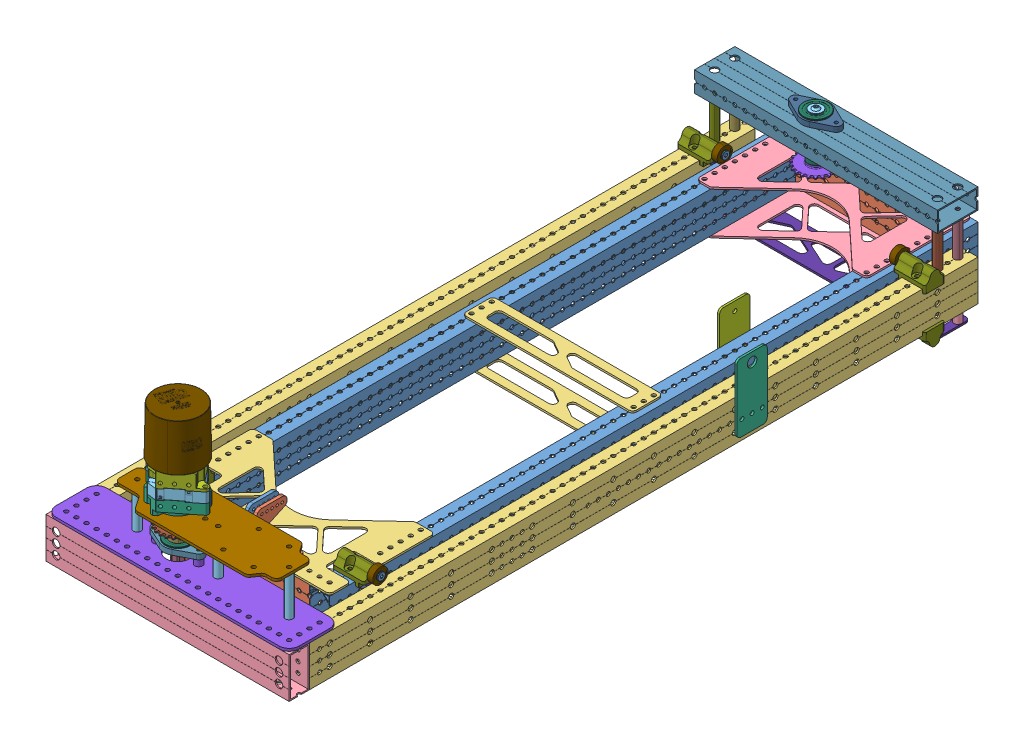
SolidWorks assembly Elevator Assembly 3.0, configuration Default. Lengths in mm. (continued)
Mates (geometry in assembly coordinates): (continued)
- Coincident51: coincident aligned: plane of WCP-EX-0018-001(2)^Assem1-1 through (-106.988 397.7257 1167.4134) normal (-1 0 0); plane of WCP-EX-0018-005(2)^Assem1-2 through (-106.988 397.7257 1116.6134) normal (-1 0 0)
- Distance1: distance = 12.7 mm anti-aligned: plane of WCP-EX-0018-005(2)^Assem1-1 through (172.412 397.7257 1116.6134) normal (-1 0 0); plane of 32inTubeStock-1 through (159.712 397.7257 265.7134) normal (1 0 0)
- Coincident53: coincident anti-aligned: plane of 32inTubeStock-1 through (159.712 448.5257 265.7134) normal (0 1 0); plane of Copy of WCP-0323 - Elevator Clamping Block-1-1/WCP-0323-001 Rev2^Copy of WCP-0323 - Elevator Clamping Block-1-1 through (159.7755 448.5257 1034.0634) normal (0 -1 0)
- Coincident57: coincident anti-aligned: plane of 7inRevTube-1 through (-43.488 448.5257 1053.1134) normal (0 1 0); plane of Inside_Bottom_Plate-1 through (-738.7858 448.5257 1008.0258) normal (0 -1 0)
- Concentric31: concentric anti-aligned: cylinder of 32inTubeStock-1 through (147.012 397.7257 1002.3134) axis (0 1 0) radius 2.5; cylinder of Inside_Bottom_Plate-1 through (147.012 450.8117 1002.3134) axis (0 -1 0) radius 2.4892
- Coincident59: coincident aligned: plane of 32inTubeStock-1 through (147.012 423.1257 1078.5134) normal (0 0 1); plane of Inside_Bottom_Plate-1 through (-738.7858 450.8117 1078.5134) normal (0 0 1)
- Concentric32: concentric anti-aligned: cylinder of 32inTubeStock-1 through (147.012 397.7257 1027.7134) axis (0 1 0) radius 2.5; cylinder of Copy of WCP-0323 - Elevator Clamping Block-1-1/WCP-0323-001 Rev2^Copy of WCP-0323 - Elevator Clamping Block-1-1 through (147.012 464.4007 1027.7134) axis (0 -1 0) radius 2.4892
- Concentric33: concentric anti-aligned: cylinder of 32inTubeStock-1 through (147.012 397.7257 1040.4134) axis (0 1 0) radius 2.5; cylinder of Copy of WCP-0323 - Elevator Clamping Block-1-1/WCP-0323-001 Rev2^Copy of WCP-0323 - Elevator Clamping Block-1-1 through (147.012 448.5257 1040.4134) axis (0 -1 0) radius 2.0193
- Concentric37: concentric anti-aligned: cylinder of 32inTubeStock-2 through (-56.188 397.7257 278.4134) axis (0 1 0) radius 2.5; cylinder of Inside_Top_Plate-1 through (-56.188 450.8117 278.4134) axis (0 -1 0) radius 2.4892
- Coincident65: coincident anti-aligned: plane of 7inRevTube-2 through (-43.488 448.5257 265.7134) normal (0 1 0); plane of Inside_Top_Plate-1 through (45.412 448.5257 384.432) normal (0 -1 0)
- Concentric38: concentric anti-aligned: cylinder of 32inTubeStock-1 through (147.012 397.7257 278.4134) axis (0 1 0) radius 2.5; cylinder of Inside_Top_Plate-1 through (147.012 450.8117 278.4134) axis (0 -1 0) radius 2.4892
- Concentric43: concentric anti-aligned: cylinder of Copy (2) of Copy of WCP-0571 Rev1^Elevator Assembly Updated 3.0-2 through (20.012 468.1632 329.2134) axis (0 1 0) radius 7.94; cylinder of Copy of Copy of WCP-0599 Rev1^Elevator Assembly Updated 3.0-1 through (20.012 469.1632 329.2134) axis (0 -1 0) radius 2.0193
- Concentric44: concentric anti-aligned: cylinder of Copy of Copy of WCP-0599 Rev1^Elevator Assembly Updated 3.0-1 through (20.012 469.1632 329.2134) axis (0 -1 0) radius 2.0193; cylinder of WCP-0790_500L_500_hex.step-1 through (20.012 478.6882 329.2134) axis (0 1 0) radius 9.75
- Concentric45: concentric anti-aligned: cylinder of Copy of Copy of WCP-0599 Rev1^Elevator Assembly 3.0-1 through (20.012 469.1632 329.2134) axis (0 -1 0) radius 2.0193; cylinder of Copy of Copy (2) of WCP-0560 Rev1^Elevator Assembly 3.0-1 through (20.012 469.1632 329.2134) axis (0 1 0) radius 9.525
- Concentric46: concentric aligned: unknown of Copy of Copy of WCP-0571 Rev1^Elevator Assembly Updated 3.0-1; cylinder of Copy of Copy of WCP-0599 Rev1^Elevator Assembly Updated 3.0-1 through (20.012 469.1632 329.2134) axis (0 -1 0) radius 2.0193
- Concentric47: concentric aligned: cylinder of WCP-0785_0_500_flanged_thunderhex_bearing.step-4 through (20.012 442.1081 329.2134) axis (0 -1 0) radius 14.2875; cylinder of Copy (2) of Copy of WCP-0476 Rev1^Elevator Assembly Updated 3.0-2 through (20.012 499.3257 329.2134) axis (0 -1 0) radius 14.2875
- Concentric48: concentric aligned: unknown of Copy (2) of Copy of WCP-0476 Rev1^Elevator Assembly Updated 3.0-2; unknown of WCP-EX-0018-002(2)^Elevator Assembly Updated 2.0-2
- Concentric49: concentric anti-aligned: cylinder of Copy (3) of Copy of WCP-0476 Rev1^Elevator Assembly Updated 3.0-3 through (45.412 524.7257 329.2134) axis (0 -1 0) radius 2.0193; unknown of WCP-EX-0018-002(2)^Elevator Assembly Updated 2.0-2
- Concentric50: concentric aligned: cylinder of WCP-0785_0_500_flanged_thunderhex_bearing.step-5 through (20.012 581.9434 329.2134) axis (0 1 0) radius 14.2875; cylinder of Copy (3) of Copy of WCP-0476 Rev1^Elevator Assembly Updated 3.0-3 through (20.012 524.7257 329.2134) axis (0 1 0) radius 14.2875
- Concentric51: concentric aligned: cylinder of WCP-0785_0_500_flanged_thunderhex_bearing.step-5 through (20.012 581.9434 329.2134) axis (0 1 0) radius 6.875; unknown of WCP-EX-0018-002(2)^Elevator Assembly Updated 2.0-2
- Concentric52: concentric anti-aligned: cylinder of WCP-0785_0_500_flanged_thunderhex_bearing.step-4 through (20.012 442.1081 329.2134) axis (0 -1 0) radius 6.875; cylinder of WCP-EX-0018-002(2)^Elevator Assembly Updated 2.0-2 through (20.012 499.3257 329.2134) axis (0 1 0) radius 12.7
- Concentric53: concentric anti-aligned: cylinder of Copy of Copy of WCP-0599 Rev1^Elevator Assembly Updated 3.0-1 through (20.012 469.1632 329.2134) axis (0 -1 0) radius 2.0193; cylinder of WCP-0785_0_500_flanged_thunderhex_bearing.step-5 through (20.012 581.9434 329.2134) axis (0 1 0) radius 6.875
- Coincident68: coincident anti-aligned: plane of WCP-0785_0_500_flanged_thunderhex_bearing.step-4 through (34.0392 492.9757 326.4989) normal (0 1 0); plane of Copy (2) of Copy of WCP-0476 Rev1^Elevator Assembly Updated 3.0-2 through (20.012 492.9757 329.2134) normal (0 -1 0)
- Coincident69: coincident aligned: unknown of Copy (3) of Copy of WCP-0207 Rev1^Elevator Assembly Updated 3.0-3; unknown of WCP-EX-0018-002(2)^Elevator Assembly Updated 2.0-2
- Coincident70: coincident anti-aligned: unknown of WCP-EX-0018-002(2)^Elevator Assembly Updated 2.0-2; unknown of Copy (4) of Copy of WCP-0207 Rev1^Elevator Assembly Updated 3.0-4
- Coincident71: coincident anti-aligned: unknown of Copy (2) of Copy of WCP-0207 Rev1^Elevator Assembly Updated 3.0-2; unknown of WCP-EX-0018-002(2)^Elevator Assembly Updated 2.0-2
- Coincident72: coincident aligned: unknown of Copy of Copy of WCP-0207 Rev1^Elevator Assembly Updated 3.0-1; cylinder of WCP-EX-0018-002(2)^Elevator Assembly Updated 2.0-2 through (185.112 512.0257 341.9134) axis (0 -1 0) radius 2.4892
- Coincident73: coincident anti-aligned: plane of WCP-EX-0018-002(2)^Elevator Assembly Updated 2.0-2 through (185.112 499.3257 303.8134) normal (0 -1 0); plane of Copy (4) of Copy of WCP-0207 Rev1^Elevator Assembly Updated 3.0-4 through (-94.288 499.3257 341.9134) normal (0 1 0)
- Coincident74: coincident anti-aligned: plane of WCP-0785_0_500_flanged_thunderhex_bearing.step-5 through (9.5354 531.0757 319.4988) normal (0 -1 0); plane of Copy (3) of Copy of WCP-0476 Rev1^Elevator Assembly Updated 3.0-3 through (20.012 531.0757 329.2134) normal (0 1 0)
- Coincident75: coincident anti-aligned: plane of Copy (2) of Copy of WCP-0571 Rev1^Elevator Assembly Updated 3.0-2 through (21.4943 469.1632 333.5519) normal (0 1 0); plane of Copy of Copy of WCP-0599 Rev1^Elevator Assembly Updated 3.0-1 through (20.012 469.1632 329.2134) normal (0 -1 0)
- Coincident76: coincident anti-aligned: plane of Copy (2) of Copy of WCP-0476 Rev1^Elevator Assembly Updated 3.0-2 through (20.012 499.3257 329.2134) normal (0 1 0); plane of WCP-EX-0018-002(2)^Elevator Assembly Updated 2.0-2 through (185.112 499.3257 303.8134) normal (0 -1 0)
- Parallel15: parallel: line of Copy of Copy of WCP-0599 Rev1^Elevator Assembly 3.0-1; line of Copy of Copy (2) of WCP-0560 Rev1^Elevator Assembly 3.0-1 through (26.8578 478.6882 331.9206) axis (-0.783433 0 0.621476)
- Coincident77: coincident aligned: plane of Copy of Copy of WCP-0599 Rev1^Elevator Assembly Updated 3.0-1 through (20.012 532.6632 329.2134) normal (0 1 0); plane of WCP-0785_0_500_flanged_thunderhex_bearing.step-5 through (12.9711 532.6632 322.6847) normal (0 1 0)
- Coincident78: coincident aligned: plane of WCP-0785_0_500_flanged_thunderhex_bearing.step-4 through (29.4391 491.3882 327.3891) normal (0 -1 0); unknown of WCP-0790_500L_500_hex.step-1
- Coincident79: coincident anti-aligned: plane of Copy of Copy (2) of WCP-0560 Rev1^Elevator Assembly 3.0-1 through (20.012 478.6882 329.2134) normal (0 1 0); plane of WCP-0790_500L_500_hex.step-1 through (20.012 478.6882 329.2134) normal (0 -1 0)
- Coincident80: coincident anti-aligned: plane of Copy of Copy of WCP-0571 Rev1^Elevator Assembly Updated 3.0-1 through (23.9967 532.6632 326.946) normal (0 -1 0); plane of Copy of Copy of WCP-0599 Rev1^Elevator Assembly Updated 3.0-1 through (20.012 532.6632 329.2134) normal (0 1 0)
- Coincident81: coincident anti-aligned: plane of Copy (2) of Copy of WCP-0571 Rev1^Elevator Assembly Updated 3.0-2 through (21.4943 469.1632 333.5519) normal (0 1 0); plane of Copy of Copy (2) of WCP-0560 Rev1^Elevator Assembly 3.0-1 through (20.012 469.1632 329.2134) normal (0 -1 0)
- Coincident82: coincident anti-aligned: plane of Copy of Copy of WCP-0207 Rev1^Elevator Assembly Updated 3.0-1 through (185.112 499.3257 341.9134) normal (0 1 0); plane of WCP-EX-0018-002(2)^Elevator Assembly Updated 2.0-2 through (185.112 499.3257 303.8134) normal (0 -1 0)
- Concentric54: concentric aligned: cylinder of WCP-EX-0018-005(2)^Assem1-1 through (185.112 397.7257 316.5134) axis (0 1 0) radius 2.4892; cylinder of WCP-EX-0018-002(2)^Elevator Assembly Updated 2.0-2 through (185.112 512.0257 316.5134) axis (0 1 0) radius 4.7625
- Concentric55: concentric aligned: cylinder of WCP-EX-0018-005(2)^Assem1-2 through (-94.288 397.7257 316.5134) axis (0 1 0) radius 2.4892; cylinder of WCP-EX-0018-002(2)^Elevator Assembly Updated 2.0-2 through (-94.288 512.0257 316.5134) axis (0 1 0) radius 4.7625
- Coincident83: coincident anti-aligned: plane of WCP-EX-0018-005(2)^Assem1-1 through (172.412 448.5257 1116.6134) normal (0 1 0); plane of Copy of Copy of WCP-0207 Rev1^Elevator Assembly Updated 3.0-1 through (185.112 448.5257 341.9134) normal (0 -1 0)
- Concentric76: concentric aligned: cylinder of REV-21-2106-universal-input-1 through (20.0926 537.3257 1129.1434) axis (0 1 0) radius 9.5504; cylinder of Neo1.1_REV-21-1650-V1.1-1 through (20.0926 552.8757 1129.1434) axis (0 1 0) radius 9.525
- Concentric77: concentric anti-aligned: cylinder of REV-21-2106-universal-input-1 through (28.0027 537.3257 1105.0064) axis (0 1 0) radius 2.5; cylinder of Neo1.1_REV-21-1650-V1.1-1 through (28.0027 556.3757 1105.0064) axis (0 -1 0) radius 2.0193
- Concentric78: concentric anti-aligned: cylinder of REV-21-2106-universal-input-1 through (12.1826 537.3257 1153.2803) axis (0 1 0) radius 2.5; cylinder of Neo1.1_REV-21-1650-V1.1-1 through (12.1826 556.3757 1153.2803) axis (0 -1 0) radius 2.0193
- Coincident109: coincident anti-aligned: plane of REV-21-2106-universal-input-1 through (20.0926 556.3757 1129.1434) normal (0 1 0); plane of Neo1.1_REV-21-1650-V1.1-1 through (20.0926 556.3757 1129.1434) normal (0 -1 0)
- Coincident116: coincident anti-aligned: plane of 32inTubeStock-2 through (-43.488 448.5257 265.7134) normal (0 1 0); plane of Copy of WCP-0323 - Elevator Clamping Block-1-9/WCP-0323-001 Rev2^Copy of WCP-0323 - Elevator Clamping Block-1-1 through (-68.9515 448.5257 1034.0634) normal (0 -1 0)
- Concentric85: concentric anti-aligned: circle of 32inTubeStock-2; cylinder of Copy of WCP-0323 - Elevator Clamping Block-1-9/WCP-0323-001 Rev2^Copy of WCP-0323 - Elevator Clamping Block-1-1 through (-56.188 464.4007 1040.4134) axis (0 -1 0) radius 2.4892
- Concentric86: concentric anti-aligned: cylinder of 32inTubeStock-2 through (-56.188 397.7257 1027.7134) axis (0 1 0) radius 2.5; cylinder of Copy of WCP-0323 - Elevator Clamping Block-1-9/WCP-0323-001 Rev2^Copy of WCP-0323 - Elevator Clamping Block-1-1 through (-56.188 448.5257 1027.7134) axis (0 -1 0) radius 2.0193
- Coincident117: coincident anti-aligned: plane of 32inTubeStock-1 through (159.712 448.5257 265.7134) normal (0 1 0); plane of Copy of WCP-0323 - Elevator Clamping Block-1-2/WCP-0323-001 Rev2^Copy of WCP-0323 - Elevator Clamping Block-1-1 through (172.3485 448.5257 360.9634) normal (0 -1 0)
- Coincident118: coincident anti-aligned: plane of 32inTubeStock-2 through (-43.488 448.5257 265.7134) normal (0 1 0); plane of Copy of WCP-0323 - Elevator Clamping Block-1-10/WCP-0323-001 Rev2^Copy of WCP-0323 - Elevator Clamping Block-1-1 through (-81.5245 448.5257 360.9634) normal (0 -1 0)
- Coincident119: coincident anti-aligned: plane of 32inTubeStock-1 through (159.712 397.7257 265.7134) normal (0 -1 0); plane of Copy of WCP-0323 - Elevator Clamping Block-1-15/WCP-0323-001 Rev2^Copy of WCP-0323 - Elevator Clamping Block-1-1 through (159.7755 397.7257 1034.0634) normal (0 1 0)
- Concentric89: concentric aligned: circle of 32inTubeStock-1; cylinder of Copy of WCP-0323 - Elevator Clamping Block-1-15/WCP-0323-001 Rev2^Copy of WCP-0323 - Elevator Clamping Block-1-1 through (147.012 381.8507 1040.4134) axis (0 1 0) radius 2.4892
- Concentric90: concentric aligned: circle of 32inTubeStock-1; cylinder of Copy of WCP-0323 - Elevator Clamping Block-1-15/WCP-0323-001 Rev2^Copy of WCP-0323 - Elevator Clamping Block-1-1 through (147.012 397.7257 1027.7134) axis (0 1 0) radius 2.0193
- Coincident120: coincident anti-aligned: plane of 32inTubeStock-1 through (159.712 397.7257 265.7134) normal (0 -1 0); plane of Copy of WCP-0323 - Elevator Clamping Block-1-16/WCP-0323-001 Rev2^Copy of WCP-0323 - Elevator Clamping Block-1-1 through (172.3485 397.7257 360.9634) normal (0 1 0)
- Coincident122: coincident anti-aligned: plane of 32inTubeStock-2 through (-43.488 397.7257 265.7134) normal (0 -1 0); plane of Copy of WCP-0323 - Elevator Clamping Block-1-17/WCP-0323-001 Rev2^Copy of WCP-0323 - Elevator Clamping Block-1-1 through (-68.9515 397.7257 1034.0634) normal (0 1 0)
- Concentric93: concentric aligned: circle of 32inTubeStock-2; circle of Copy of WCP-0323 - Elevator Clamping Block-1-17/WCP-0323-001 Rev2^Copy of WCP-0323 - Elevator Clamping Block-1-1
- Concentric94: concentric aligned: circle of 32inTubeStock-2; circle of Copy of WCP-0323 - Elevator Clamping Block-1-17/WCP-0323-001 Rev2^Copy of WCP-0323 - Elevator Clamping Block-1-1
- Coincident126: coincident anti-aligned: plane of 32inTubeStock-2 through (-43.488 397.7257 265.7134) normal (0 -1 0); plane of Copy of WCP-0323 - Elevator Clamping Block-1-18/WCP-0323-001 Rev2^Copy of WCP-0323 - Elevator Clamping Block-1-1 through (-81.5245 397.7257 360.9634) normal (0 1 0)
- Coincident127: coincident anti-aligned: plane of 7inRevTube-1 through (-43.488 397.7257 1053.1134) normal (0 -1 0); plane of Inside_Bottom_Plate-3 through (-738.7858 397.7257 1008.0258) normal (0 1 0)
- Concentric97: concentric anti-aligned: cylinder of 32inTubeStock-1 through (147.012 397.7257 1065.8134) axis (0 1 0) radius 2.5; circle of Part1^Elevator Assembly Updated 3.0-3
- Concentric98: concentric anti-aligned: cylinder of 32inTubeStock-1 through (147.012 397.7257 1002.3134) axis (0 1 0) radius 2.5; cylinder of Inside_Bottom_Plate-3 through (147.012 397.7257 1002.3134) axis (0 -1 0) radius 2.4892
- Coincident143: coincident anti-aligned: plane of Inside_Bottom_Plate-1 through (-738.7858 450.8117 1008.0258) normal (0 1 0); plane of WCP-0583-026 Rev1.step-1 through (77.162 450.8117 1065.8134) normal (0 -1 0)
- Coincident144: coincident anti-aligned: plane of Inside_Bottom_Plate-1 through (-738.7858 450.8117 1008.0258) normal (0 1 0); plane of WCP-0583-025 Rev1_DefaultSM-FLAT-PATTERN.step-1 through (23.187 450.8117 1065.8134) normal (0 -1 0)
- Coincident145: coincident anti-aligned: cylinder of Inside_Bottom_Plate-1 through (70.812 450.8117 1065.8134) axis (0 -1 0) radius 2.4892; circle of WCP-0583-026 Rev1.step-1
- Concentric111: concentric anti-aligned: cylinder of Inside_Bottom_Plate-1 through (96.212 450.8117 1065.8134) axis (0 -1 0) radius 2.4892; cylinder of WCP-0583-026 Rev1.step-1 through (96.212 450.8117 1065.8134) axis (0 1 0) radius 2.4892
- Coincident146: coincident aligned: circle of Part1^Elevator Assembly Updated 3.0-1; cylinder of WCP-0583-025 Rev1_DefaultSM-FLAT-PATTERN.step-1 through (32.712 450.8117 1065.8134) axis (0 1 0) radius 2.4892
- Concentric112: concentric anti-aligned: cylinder of Inside_Bottom_Plate-1 through (7.312 450.8117 1065.8134) axis (0 -1 0) radius 2.4892; cylinder of WCP-0583-025 Rev1_DefaultSM-FLAT-PATTERN.step-1 through (7.312 450.8117 1065.8134) axis (0 1 0) radius 2.4892
- InPlace4: in place: plane of ? through (-43.488 448.5257 147.5168) normal (0 1 0); plane of ? through (0 448.5257 0) normal (0 1 0); moOrthogonalPlaneRef_w of ? through (-43.488 448.5257 147.5168) normal (0 1 0); plane of ? through (0 448.5257 0) normal (0 0 -1); plane of ? through (-43.488 448.5257 147.5168) normal (0 1 0); plane of ? through (0 448.5257 0) normal (1 0 0); plane of 32inTubeStock-2 through (-43.488 448.5257 265.7134) normal (0 1 0); unknown of Inside_Middle_Plate-1
- Coincident147: coincident aligned: 
- Coincident148: coincident aligned: plane of 32inTubeStock-2 through (-56.188 448.5257 1446.8134) normal (0 0 -1); plane of Inside_Middle_Plate-1 through (-56.188 448.5257 1446.8134) normal (0 0 -1)
- Coincident149: coincident anti-aligned: plane of 32inTubeStock-2 through (-56.188 448.5257 1446.8134) normal (-1 0 0); plane of Inside_Middle_Plate-1 through (-56.188 448.5257 1446.8134) normal (1 0 0)
- Coincident150: coincident anti-aligned: plane of 32inTubeStock-2 through (-43.488 397.7257 265.7134) normal (0 -1 0); plane of Inside_Middle_Plate-2 through (154.632 397.7257 658.1434) normal (0 1 0)
- Concentric113: concentric aligned: cylinder of Inside_Middle_Plate-1 through (-56.188 450.8117 684.8134) axis (0 -1 0) radius 2.5; cylinder of Inside_Middle_Plate-2 through (-56.188 397.7257 684.8134) axis (0 -1 0) radius 2.5
- Concentric114: concentric aligned: cylinder of Inside_Middle_Plate-1 through (-56.188 450.8117 659.4134) axis (0 -1 0) radius 2.5; cylinder of Inside_Middle_Plate-2 through (-56.188 397.7257 659.4134) axis (0 -1 0) radius 2.5
- Coincident154: coincident aligned: plane of 0_750_L_10_thru_WCP-0217-1 through (-94.288 397.7257 341.9134) normal (0 1 0); plane of 0_750_L_10_thru_WCP-0217-5 through (185.112 397.7257 316.5134) normal (0 1 0)
- Concentric115: concentric anti-aligned: cylinder of WCP-EX-0018-005(2)^Assem1-1 through (185.112 397.7257 316.5134) axis (0 1 0) radius 2.4892; cylinder of 0_750_L_10_thru_WCP-0217-5 through (185.112 397.7257 316.5134) axis (0 -1 0) radius 2.4892
- Coincident156: coincident anti-aligned: plane of WCP-EX-0018-005(2)^Assem1-1 through (172.412 397.7257 1116.6134) normal (0 -1 0); plane of 0_750_L_10_thru_WCP-0217-5 through (185.112 397.7257 316.5134) normal (0 1 0)
- Concentric116: concentric anti-aligned: cylinder of WCP-EX-0018-005(2)^Assem1-1 through (185.112 397.7257 341.9134) axis (0 1 0) radius 2.4892; cylinder of 0_750_L_10_thru_WCP-0217-3 through (185.112 397.7257 341.9134) axis (0 -1 0) radius 2.4892
- Concentric117: concentric anti-aligned: cylinder of WCP-EX-0018-005(2)^Assem1-2 through (-94.288 397.7257 316.5134) axis (0 1 0) radius 2.4892; cylinder of 0_750_L_10_thru_WCP-0217-2 through (-94.288 397.7257 316.5134) axis (0 -1 0) radius 2.4892
- Concentric118: concentric anti-aligned: cylinder of 0_750_L_10_thru_WCP-0217-1 through (-94.288 397.7257 341.9134) axis (0 -1 0) radius 2.4892; cylinder of WCP-EX-0018-005(2)^Assem1-2 through (-94.288 397.7257 341.9134) axis (0 1 0) radius 2.4892
- Coincident158: coincident anti-aligned: plane of 32inTubeStock-2 through (-43.488 397.7257 265.7134) normal (0 -1 0); plane of Inside_Top_Plate-2 through (45.412 397.7257 384.432) normal (0 1 0)
- Concentric119: concentric anti-aligned: cylinder of 32inTubeStock-2 through (-56.188 397.7257 278.4134) axis (0 1 0) radius 2.5; cylinder of Inside_Top_Plate-2 through (-56.188 397.7257 278.4134) axis (0 -1 0) radius 2.4892
- Concentric120: concentric anti-aligned: cylinder of 32inTubeStock-1 through (147.012 397.7257 278.4134) axis (0 1 0) radius 2.5; cylinder of Inside_Top_Plate-2 through (147.012 397.7257 278.4134) axis (0 -1 0) radius 2.4892
- Coincident160: coincident aligned: plane of 2_000_L_10_thru_WCP-0207-1 through (70.8227 451.7007 1129.3134) normal (0 -1 0); plane of 2_000_L_10_thru_WCP-0207-2 through (-30.7773 451.7007 1129.3134) normal (0 -1 0)
- Coincident173: coincident aligned: circle of Outside_Top_Plate-1; cylinder of 0_750_L_10_thru_WCP-0217-2 through (-94.288 397.7257 316.5134) axis (0 -1 0) radius 2.4892
- Concentric133: concentric anti-aligned: cylinder of Outside_Top_Plate-1 through (-94.288 376.3897 341.9134) axis (0 1 0) radius 2.4892; cylinder of 0_750_L_10_thru_WCP-0217-1 through (-94.288 397.7257 341.9134) axis (0 -1 0) radius 2.4892
- Coincident174: coincident anti-aligned: plane of Outside_Top_Plate-1 through (185.112 378.6757 316.5134) normal (0 1 0); plane of 0_750_L_10_thru_WCP-0217-1 through (-94.288 378.6757 341.9134) normal (0 -1 0)
- Coincident175: coincident anti-aligned: plane of WCP-EX-0018-005(2)^Assem1-2 through (-106.988 397.7257 1116.6134) normal (0 -1 0); plane of 0_750_L_10_thru_WCP-0217-2 through (-94.288 397.7257 316.5134) normal (0 1 0)
- Coincident176: coincident anti-aligned: plane of WCP-EX-0018-005(2)^Assem1-1 through (172.412 397.7257 1116.6134) normal (0 -1 0); plane of 0_750_L_10_thru_WCP-0217-3 through (185.112 397.7257 341.9134) normal (0 1 0)
- Concentric134: concentric anti-aligned: cylinder of WCP-EX-0018-005(2)^Assem1-2 through (-94.288 397.7257 354.6134) axis (0 1 0) radius 2.4892; cylinder of Copy of WCP-0323 - Elevator Clamping Block-1-10/WCP-0323-001 Rev2^Copy of WCP-0323 - Elevator Clamping Block-1-1 through (-94.288 464.4007 354.6134) axis (0 -1 0) radius 2.4892
- Concentric135: concentric anti-aligned: cylinder of WCP-EX-0018-005(2)^Assem1-2 through (-94.288 397.7257 367.3134) axis (0 1 0) radius 2.4892; cylinder of Copy of WCP-0323 - Elevator Clamping Block-1-10/WCP-0323-001 Rev2^Copy of WCP-0323 - Elevator Clamping Block-1-1 through (-94.288 448.5257 367.3134) axis (0 -1 0) radius 2.0193
- Concentric136: concentric aligned: circle of WCP-EX-0018-005(2)^Assem1-1; circle of Copy of WCP-0323 - Elevator Clamping Block-1-2/WCP-0323-001 Rev2^Copy of WCP-0323 - Elevator Clamping Block-1-1
- Concentric137: concentric anti-aligned: circle of WCP-EX-0018-005(2)^Assem1-1; cylinder of Copy of WCP-0323 - Elevator Clamping Block-1-2/WCP-0323-001 Rev2^Copy of WCP-0323 - Elevator Clamping Block-1-1 through (185.112 448.5257 354.6134) axis (0 -1 0) radius 2.0193
- Concentric138: concentric aligned: circle of WCP-EX-0018-005(2)^Assem1-2; circle of Copy of WCP-0323 - Elevator Clamping Block-1-18/WCP-0323-001 Rev2^Copy of WCP-0323 - Elevator Clamping Block-1-1
- Concentric139: concentric aligned: cylinder of WCP-EX-0018-005(2)^Assem1-2 through (-94.288 397.7257 367.3134) axis (0 1 0) radius 2.4892; cylinder of Copy of WCP-0323 - Elevator Clamping Block-1-18/WCP-0323-001 Rev2^Copy of WCP-0323 - Elevator Clamping Block-1-1 through (-94.288 381.8507 367.3134) axis (0 1 0) radius 2.4892
- Concentric140: concentric aligned: circle of WCP-EX-0018-005(2)^Assem1-1; circle of Copy of WCP-0323 - Elevator Clamping Block-1-16/WCP-0323-001 Rev2^Copy of WCP-0323 - Elevator Clamping Block-1-1
- Concentric141: concentric aligned: circle of WCP-EX-0018-005(2)^Assem1-1; cylinder of Copy of WCP-0323 - Elevator Clamping Block-1-16/WCP-0323-001 Rev2^Copy of WCP-0323 - Elevator Clamping Block-1-1 through (185.112 381.8507 354.6134) axis (0 1 0) radius 2.4892
- Coincident179: coincident anti-aligned: plane of Motor_Mounting_Plate-1 through (-30.7773 502.5007 1129.3134) normal (0 -1 0); plane of 2_000_L_10_thru_WCP-0207-1 through (70.8227 502.5007 1129.3134) normal (0 1 0)
- Concentric152: concentric anti-aligned: circle of Motor_Mounting_Plate-1; cylinder of 2_000_L_10_thru_WCP-0207-1 through (70.8227 451.7007 1129.3134) axis (0 1 0) radius 2.4892
- Concentric153: concentric anti-aligned: cylinder of Motor_Mounting_Plate-1 through (-30.7773 502.5007 1129.3134) axis (0 1 0) radius 2.54; circle of 2_000_L_10_thru_WCP-0207-2
- Coincident180: coincident anti-aligned: plane of REV-21-2104-hex-socket-output-1 through (20.0961 505.6757 1129.1406) normal (0 -1 0); plane of Motor_Mounting_Plate-1 through (-30.7773 505.6757 1129.3134) normal (0 1 0)
- Angle6: planar angle = 0.316585 rad aligned: plane of REV-21-2104-hex-socket-output-1 through (24.3674 524.7257 1093.4744) normal (-0.61801 0 -0.78617); plane of Motor_Mounting_Plate-1 through (-11.7273 502.5007 1113.4384) normal (-0.83205 0 -0.5547)
- Concentric159: concentric anti-aligned: cylinder of Motor_Mounting_Plate-1 through (159.7227 357.5593 1129.3134) axis (0 1 0) radius 2.54; circle of 2_000_L_10_thru_WCP-0207-3
- Coincident182: coincident anti-aligned: plane of Motor_Mounting_Plate-1 through (-30.7773 502.5007 1129.3134) normal (0 -1 0); plane of 2_000_L_10_thru_WCP-0207-3 through (159.7227 502.5007 1129.3134) normal (0 1 0)
- Concentric160: concentric anti-aligned: cylinder of WCP-EX-0018-005(2)^Assem1-1 through (172.412 423.1257 589.5634) axis (1 0 0) radius 2.4892; cylinder of Part5^Elevator Assembly 3.0-1 through (200.352 423.1257 589.5634) axis (-1 0 0) radius 2.4892
- Concentric161: concentric anti-aligned: cylinder of WCP-EX-0018-005(2)^Assem1-1 through (172.412 423.1257 576.8634) axis (1 0 0) radius 2.4892; cylinder of Part5^Elevator Assembly 3.0-1 through (200.352 423.1257 576.8634) axis (-1 0 0) radius 2.4892
- Coincident187: coincident anti-aligned: plane of WCP-EX-0018-005(2)^Assem1-1 through (197.812 397.7257 1116.6134) normal (1 0 0); plane of Part5^Elevator Assembly 3.0-1 through (197.812 409.1557 575.5934) normal (-1 0 0)
- Coincident188: coincident anti-aligned: plane of 32inTubeStock-1 through (134.312 397.7257 265.7134) normal (-1 0 0); plane of Copy of Part5^Elevator Assembly 3.0-1 through (134.312 409.1557 531.1434) normal (1 0 0)
- Concentric164: concentric anti-aligned: circle of 32inTubeStock-1; cylinder of Copy of Part5^Elevator Assembly 3.0-1 through (134.312 423.1257 532.4134) axis (-1 0 0) radius 2.4892
- Concentric165: concentric anti-aligned: cylinder of 32inTubeStock-1 through (159.712 423.1257 557.8134) axis (1 0 0) radius 2.5; cylinder of Copy of Part5^Elevator Assembly 3.0-1 through (134.312 423.1257 557.8134) axis (-1 0 0) radius 2.4892
- Coincident189: coincident anti-aligned: plane of WCP-EX-0018-001(2)^Assem1-1 through (235.912 448.5257 1167.4134) normal (0 1 0); plane of New_Motor_Mounting_Plate-1 through (197.812 448.5257 1103.9134) normal (0 -1 0)
- Coincident190: coincident aligned: plane of WCP-EX-0018-001(2)^Assem1-1 through (235.912 397.7257 1167.4134) normal (0 0 1); plane of New_Motor_Mounting_Plate-1 through (197.812 451.7007 1167.4134) normal (0 0 1)
- Coincident191: coincident aligned: plane of WCP-EX-0018-005(2)^Assem1-2 through (-106.988 397.7257 1116.6134) normal (-1 0 0); plane of New_Motor_Mounting_Plate-1 through (-106.988 451.7007 1103.9134) normal (-1 0 0)
- Distance2: distance = 88.9 mm aligned: plane of WCP-EX-0018-001(2)^Assem1-1 through (235.912 397.7257 1167.4134) normal (0 0 1); plane of 7inRevTube-1 through (-43.488 397.7257 1078.5134) normal (0 0 1)
- Concentric166: concentric aligned: cylinder of 2_000_L_10_thru_WCP-0207-3 through (159.7227 451.7007 1129.3134) axis (0 1 0) radius 4.7498; cylinder of New_Motor_Mounting_Plate-1 through (159.7227 448.5257 1129.3134) axis (0 1 0) radius 2.4892
- Coincident193: coincident anti-aligned: plane of 2_000_L_10_thru_WCP-0207-2 through (-30.7773 451.7007 1129.3134) normal (0 -1 0); plane of New_Motor_Mounting_Plate-1 through (197.812 451.7007 1103.9134) normal (0 1 0)
- Concentric168: concentric aligned: cylinder of 2_000_L_10_thru_WCP-0207-2 through (-30.7773 451.7007 1129.3134) axis (0 1 0) radius 4.7498; cylinder of New_Motor_Mounting_Plate-1 through (-30.7773 448.5257 1129.3134) axis (0 1 0) radius 2.4892
- Coincident194: coincident anti-aligned: plane of Copy (3) of Copy of WCP-0308 Rev1^Elevator Assembly 3.0-4 through (-5.2931 451.7007 1129.8798) normal (0 -1 0); plane of New_Motor_Mounting_Plate-1 through (197.812 451.7007 1103.9134) normal (0 1 0)
- Concentric169: concentric anti-aligned: cylinder of REV-21-2106-universal-input-1 through (54.5541 537.3257 1129.3134) axis (0 1 0) radius 2.5; cylinder of Motor_Mounting_Plate-1 through (54.5541 505.6757 1129.3134) axis (0 -1 0) radius 2.54
- Concentric170: concentric anti-aligned: cylinder of Copy of Copy of WCP-0789_250L_500_hex^Elevator Assembly 3.0-1 through (20.0961 474.6242 1129.1406) axis (0 -1 0) radius 9.75; cylinder of 0_125_L_500_hex_spacer_217-2758-2 through (20.0961 474.6242 1129.1406) axis (0 1 0) radius 9.525
- Coincident195: coincident anti-aligned: plane of Copy of Copy of WCP-0789_250L_500_hex^Elevator Assembly 3.0-1 through (20.0961 474.6242 1129.1406) normal (0 1 0); circle of 0_125_L_500_hex_spacer_217-2758-2
- Parallel16: parallel anti-aligned: plane of 1_2ThunderHex-1 through (27.0889 1329.5882 1126.8394) normal (0.666327 0 -0.74566); plane of 0_125_L_500_hex_spacer_217-2758-2 through (21.6235 474.6242 1121.8192) normal (-0.666327 0 0.74566)
- Coincident197: coincident anti-aligned: plane of Copy of Copy of WCP-0560 Rev1^Elevator Assembly 3.0-1 through (20.0961 477.7992 1129.1406) normal (0 -1 0); plane of 0_125_L_500_hex_spacer_217-2758-2 through (20.0961 477.7992 1129.1406) normal (0 1 0)
